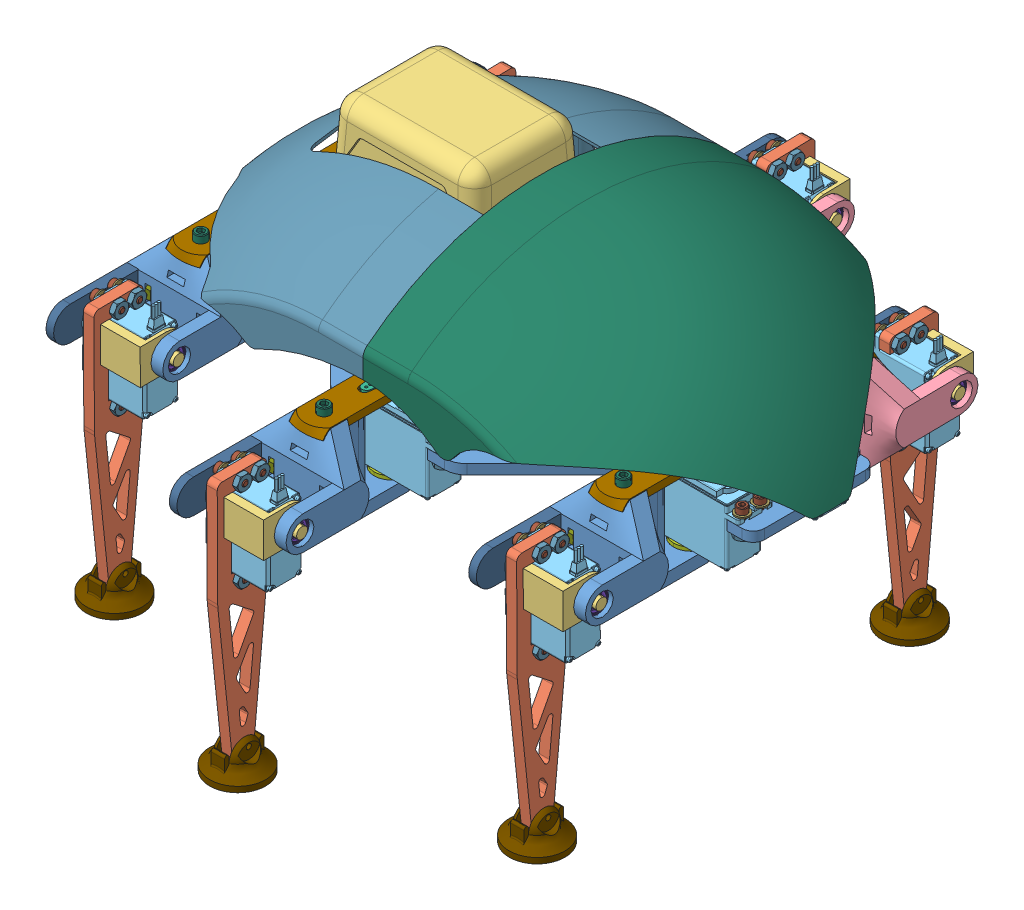
SolidWorks assembly Hexapod_(Leg_V1+Body_V2), configuration Défaut. Lengths in mm. (continued)
Components (placement in the parent): (continued)
- Battery-1: Battery [Défaut] at (-118.1821 62.8376 15.5603) x (0 0 -1) z (-1 0 0) size (64.47 74.3 85.78)
  - MAKITA 4.0AH-1: MAKITA 4.0AH [Défaut] at (0.5853 -29.7874 85.4436) size (64.47 57.15 85.78)
  - MAKITA 4.0AH MOBILE-1: MAKITA 4.0AH MOBILE [Défaut] at (0.5853 -39.3124 91.7936) size (45.84 26.68 66.29)
- arduinoMega-1: arduinoMega [Detailed] at (-199.11 -7.6 14.62) x (0 0 -1) z (-1 0 0) size (108.32 14.5 53.3)
- raspberryPi3B-1: raspberryPi3B [Detailed] at (-109 6.35 15) x (-1 0 0) z (0 1 0) size (87.05 58.5 19.5)
- 12Channel PWM-1: 12Channel PWM [Default] at (-145.6 -5.6 15) x (-1 0 0) z (0 0 1) size (25.4 7.55 66.7)
- DROK_090483.stp-1: DROK_090483.stp [Default] at (-77.5 -5.6 45) x (-1 0 0) z (0 -1 0) size (50.02 60 18.9)
- HX-SHCS 0.138-32x0.625x0.625-N-2: HX-SHCS 0.138-32x0.625x0.625-N [HX-SHCS 0.138-32x0.625x0.625-N] at (-40.288 3.5052 19.09) x (0 -1 0) z (1 0 0) size (19.38 5.74 5.74)
- HX-SHCS 0.138-32x0.625x0.625-N-3: HX-SHCS 0.138-32x0.625x0.625-N [HX-SHCS 0.138-32x0.625x0.625-N] at (-50.288 3.5052 19.09) x (0 -1 0) z (0.5 0 0.866025) size (19.38 5.74 5.74)
- HX-SHCS 0.138-32x0.625x0.625-N-4: HX-SHCS 0.138-32x0.625x0.625-N [HX-SHCS 0.138-32x0.625x0.625-N] at (-50.288 3.5052 10.91) x (0 -1 0) z (1 0 0) size (19.38 5.74 5.74)
- HX-SHCS 0.138-32x0.625x0.625-N-5: HX-SHCS 0.138-32x0.625x0.625-N [HX-SHCS 0.138-32x0.625x0.625-N] at (-40.288 3.5052 10.91) x (0 -1 0) z (1 0 0) size (19.38 5.74 5.74)
- HX-SHCS 0.138-32x0.625x0.625-N-6: HX-SHCS 0.138-32x0.625x0.625-N [HX-SHCS 0.138-32x0.625x0.625-N] at (-170.288 3.5052 69.09) x (0 -1 0) z (1 0 0) size (19.38 5.74 5.74)
- HX-SHCS 0.138-32x0.625x0.625-N-7: HX-SHCS 0.138-32x0.625x0.625-N [HX-SHCS 0.138-32x0.625x0.625-N] at (-160.288 3.5052 69.09) x (0 -1 0) z (1 0 0) size (19.38 5.74 5.74)
- HX-SHCS 0.138-32x0.625x0.625-N-14: HX-SHCS 0.138-32x0.625x0.625-N [HX-SHCS 0.138-32x0.625x0.625-N] at (-160.288 3.5052 -39.09) x (0 -1 0) z (1 0 0) size (19.38 5.74 5.74)
- HX-SHCS 0.138-32x0.625x0.625-N-15: HX-SHCS 0.138-32x0.625x0.625-N [HX-SHCS 0.138-32x0.625x0.625-N] at (-170.288 3.5052 -39.09) x (0 -1 0) z (1 0 0) size (19.38 5.74 5.74)
- HX-SHCS 0.138-32x0.625x0.625-N-16: HX-SHCS 0.138-32x0.625x0.625-N [HX-SHCS 0.138-32x0.625x0.625-N] at (-280.288 3.5052 19.09) x (0 -1 0) z (1 0 0) size (19.38 5.74 5.74)
- HX-SHCS 0.138-32x0.625x0.625-N-17: HX-SHCS 0.138-32x0.625x0.625-N [HX-SHCS 0.138-32x0.625x0.625-N] at (-290.288 3.5052 19.09) x (0 -1 0) z (0.5 0 0.866025) size (19.38 5.74 5.74)
- HX-SHCS 0.138-32x0.625x0.625-N-18: HX-SHCS 0.138-32x0.625x0.625-N [HX-SHCS 0.138-32x0.625x0.625-N] at (-290.288 3.5052 10.91) x (0 -1 0) z (1 0 0) size (19.38 5.74 5.74)
- HX-SHCS 0.138-32x0.625x0.625-N-19: HX-SHCS 0.138-32x0.625x0.625-N [HX-SHCS 0.138-32x0.625x0.625-N] at (-280.288 3.5052 10.91) x (0 -1 0) z (1 0 0) size (19.38 5.74 5.74)
- MSHXNUT 0.138-32-D-N-60: MSHXNUT 0.138-32-D-N [MSHXNUT 0.138-32-D-N] at (-298.75 -8.4956 -15.08) x (1 0 0) z (0 -1 0) size (7.92 9.15 2.9)
- MSHXNUT 0.138-32-D-N-65: MSHXNUT 0.138-32-D-N [MSHXNUT 0.138-32-D-N] at (-298.75 -8.4956 -4.92) x (1 0 0) z (0 -1 0) size (7.92 9.15 2.9)
- MSHXNUT 0.138-32-D-N-70: MSHXNUT 0.138-32-D-N [MSHXNUT 0.138-32-D-N] at (-251.252 -8.4956 -4.92) x (0.5 0 0.866025) z (0 -1 0) size (7.92 9.15 2.9)
- MSHXNUT 0.138-32-D-N-75: MSHXNUT 0.138-32-D-N [MSHXNUT 0.138-32-D-N] at (-251.252 -8.4956 -15.08) x (0.5 0 0.866025) z (0 -1 0) size (7.92 9.15 2.9)
- MSHXNUT 0.138-32-D-N-80: MSHXNUT 0.138-32-D-N [MSHXNUT 0.138-32-D-N] at (-280.288 -13.5656 10.91) x (0 0 1) z (0 -1 0) size (7.92 9.15 2.9)
- MSHXNUT 0.138-32-D-N-85: MSHXNUT 0.138-32-D-N [MSHXNUT 0.138-32-D-N] at (-290.288 -13.5656 10.91) x (0 0 1) z (0 -1 0) size (7.92 9.15 2.9)
- MSHXNUT 0.138-32-D-N-88: MSHXNUT 0.138-32-D-N [MSHXNUT 0.138-32-D-N] at (-178.75 -8.4956 -65.08) x (1 0 0) z (0 -1 0) size (7.92 9.15 2.9)
- MSHXNUT 0.138-32-D-N-89: MSHXNUT 0.138-32-D-N [MSHXNUT 0.138-32-D-N] at (-178.75 -8.4956 -54.92) x (1 0 0) z (0 -1 0) size (7.92 9.15 2.9)
- MSHXNUT 0.138-32-D-N-90: MSHXNUT 0.138-32-D-N [MSHXNUT 0.138-32-D-N] at (-131.252 -8.4956 -54.92) x (0.5 0 0.866025) z (0 -1 0) size (7.92 9.15 2.9)
- MSHXNUT 0.138-32-D-N-91: MSHXNUT 0.138-32-D-N [MSHXNUT 0.138-32-D-N] at (-131.252 -8.4956 -65.08) x (0.5 0 0.866025) z (0 -1 0) size (7.92 9.15 2.9)
- MSHXNUT 0.138-32-D-N-92: MSHXNUT 0.138-32-D-N [MSHXNUT 0.138-32-D-N] at (-160.288 -13.5656 -39.09) x (0 0 1) z (0 -1 0) size (7.92 9.15 2.9)
- MSHXNUT 0.138-32-D-N-93: MSHXNUT 0.138-32-D-N [MSHXNUT 0.138-32-D-N] at (-170.288 -13.5656 -39.09) x (0 0 1) z (0 -1 0) size (7.92 9.15 2.9)
- MSHXNUT 0.138-32-D-N-94: MSHXNUT 0.138-32-D-N [MSHXNUT 0.138-32-D-N] at (-50.288 -13.5656 10.91) x (0 0 1) z (0 -1 0) size (7.92 9.15 2.9)
- MSHXNUT 0.138-32-D-N-95: MSHXNUT 0.138-32-D-N [MSHXNUT 0.138-32-D-N] at (-40.288 -13.5656 10.91) x (0 0 1) z (0 -1 0) size (7.92 9.15 2.9)
- MSHXNUT 0.138-32-D-N-96: MSHXNUT 0.138-32-D-N [MSHXNUT 0.138-32-D-N] at (-11.252 -8.4956 -4.92) x (0.5 0 0.866025) z (0 -1 0) size (7.92 9.15 2.9)
- MSHXNUT 0.138-32-D-N-97: MSHXNUT 0.138-32-D-N [MSHXNUT 0.138-32-D-N] at (-11.252 -8.4956 -15.08) x (0.5 0 0.866025) z (0 -1 0) size (7.92 9.15 2.9)
- MSHXNUT 0.138-32-D-N-98: MSHXNUT 0.138-32-D-N [MSHXNUT 0.138-32-D-N] at (-58.75 -8.4956 -4.92) x (1 0 0) z (0 -1 0) size (7.92 9.15 2.9)
- MSHXNUT 0.138-32-D-N-99: MSHXNUT 0.138-32-D-N [MSHXNUT 0.138-32-D-N] at (-58.75 -8.4956 -15.08) x (1 0 0) z (0 -1 0) size (7.92 9.15 2.9)
- MSHXNUT 0.138-32-D-N-100: MSHXNUT 0.138-32-D-N [MSHXNUT 0.138-32-D-N] at (-290.288 -10.67 19.09) x (0 0 -1) z (0 1 0) size (7.92 9.15 2.9)
- MSHXNUT 0.138-32-D-N-101: MSHXNUT 0.138-32-D-N [MSHXNUT 0.138-32-D-N] at (-280.288 -10.67 19.09) x (0 0 -1) z (0 1 0) size (7.92 9.15 2.9)
- MSHXNUT 0.138-32-D-N-102: MSHXNUT 0.138-32-D-N [MSHXNUT 0.138-32-D-N] at (-251.252 -5.6 34.92) x (0.5 0 -0.866025) z (0 1 0) size (7.92 9.15 2.9)
- MSHXNUT 0.138-32-D-N-103: MSHXNUT 0.138-32-D-N [MSHXNUT 0.138-32-D-N] at (-251.252 -5.6 45.08) x (0.5 0 -0.866025) z (0 1 0) size (7.92 9.15 2.9)
- MSHXNUT 0.138-32-D-N-104: MSHXNUT 0.138-32-D-N [MSHXNUT 0.138-32-D-N] at (-298.75 -5.6 34.92) x (1 0 0) z (0 1 0) size (7.92 9.15 2.9)
- MSHXNUT 0.138-32-D-N-105: MSHXNUT 0.138-32-D-N [MSHXNUT 0.138-32-D-N] at (-298.75 -5.6 45.08) x (1 0 0) z (0 1 0) size (7.92 9.15 2.9)
- MSHXNUT 0.138-32-D-N-106: MSHXNUT 0.138-32-D-N [MSHXNUT 0.138-32-D-N] at (-178.75 -5.6 95.08) x (1 0 0) z (0 1 0) size (7.92 9.15 2.9)
- MSHXNUT 0.138-32-D-N-107: MSHXNUT 0.138-32-D-N [MSHXNUT 0.138-32-D-N] at (-178.75 -5.6 84.92) x (1 0 0) z (0 1 0) size (7.92 9.15 2.9)
- MSHXNUT 0.138-32-D-N-108: MSHXNUT 0.138-32-D-N [MSHXNUT 0.138-32-D-N] at (-131.252 -5.6 84.92) x (0.5 0 -0.866025) z (0 1 0) size (7.92 9.15 2.9)
- MSHXNUT 0.138-32-D-N-109: MSHXNUT 0.138-32-D-N [MSHXNUT 0.138-32-D-N] at (-131.252 -5.6 95.08) x (0.5 0 -0.866025) z (0 1 0) size (7.92 9.15 2.9)
- MSHXNUT 0.138-32-D-N-110: MSHXNUT 0.138-32-D-N [MSHXNUT 0.138-32-D-N] at (-160.288 -10.67 69.09) x (0 0 -1) z (0 1 0) size (7.92 9.15 2.9)
- MSHXNUT 0.138-32-D-N-111: MSHXNUT 0.138-32-D-N [MSHXNUT 0.138-32-D-N] at (-170.288 -10.67 69.09) x (0 0 -1) z (0 1 0) size (7.92 9.15 2.9)
- MSHXNUT 0.138-32-D-N-112: MSHXNUT 0.138-32-D-N [MSHXNUT 0.138-32-D-N] at (-50.288 -10.67 19.09) x (0 0 -1) z (0 1 0) size (7.92 9.15 2.9)
- MSHXNUT 0.138-32-D-N-113: MSHXNUT 0.138-32-D-N [MSHXNUT 0.138-32-D-N] at (-40.288 -10.67 19.09) x (0 0 -1) z (0 1 0) size (7.92 9.15 2.9)
- MSHXNUT 0.138-32-D-N-114: MSHXNUT 0.138-32-D-N [MSHXNUT 0.138-32-D-N] at (-11.252 -5.6 34.92) x (0.5 0 -0.866025) z (0 1 0) size (7.92 9.15 2.9)
- MSHXNUT 0.138-32-D-N-115: MSHXNUT 0.138-32-D-N [MSHXNUT 0.138-32-D-N] at (-11.252 -5.6 45.08) x (0.5 0 -0.866025) z (0 1 0) size (7.92 9.15 2.9)
- MSHXNUT 0.138-32-D-N-116: MSHXNUT 0.138-32-D-N [MSHXNUT 0.138-32-D-N] at (-58.75 -5.6 34.92) x (1 0 0) z (0 1 0) size (7.92 9.15 2.9)
- MSHXNUT 0.138-32-D-N-117: MSHXNUT 0.138-32-D-N [MSHXNUT 0.138-32-D-N] at (-58.75 -5.6 45.08) x (1 0 0) z (0 1 0) size (7.92 9.15 2.9)
- HX-SHCS 0.138-32x0.5x0.5-N-20: HX-SHCS 0.138-32x0.5x0.5-N [HX-SHCS 0.138-32x0.5x0.5-N] at (-175 -12.6052 48.88) x (0 1 0) z (-0.5 0 -0.866025) size (16.21 5.74 5.74)
- HX-SHCS 0.138-32x0.5x0.5-N-21: HX-SHCS 0.138-32x0.5x0.5-N [HX-SHCS 0.138-32x0.5x0.5-N] at (-223.22 -12.6052 -32.36) x (0 1 0) z (1 0 0) size (16.21 5.74 5.74)
- HX-SHCS 0.138-32x0.5x0.5-N-22: HX-SHCS 0.138-32x0.5x0.5-N [HX-SHCS 0.138-32x0.5x0.5-N] at (-175 -12.6052 -26) x (0 1 0) z (-0.5 0 -0.866025) size (16.21 5.74 5.74)
- HX-SHCS 0.138-32x0.5x0.5-N-23: HX-SHCS 0.138-32x0.5x0.5-N [HX-SHCS 0.138-32x0.5x0.5-N] at (-223.22 -12.6052 50.11) x (0 1 0) z (-1 0 0) size (16.21 5.74 5.74)
- MSHXNUT 0.112-40-D-N-106: MSHXNUT 0.112-40-D-N [MSHXNUT 0.112-40-D-N] at (-223.22 2.4892 -32.36) x (1 0 0) z (0 1 0) size (6.35 7.33 2.49)
- MSHXNUT 0.112-40-D-N-107: MSHXNUT 0.112-40-D-N [MSHXNUT 0.112-40-D-N] at (-223.22 2.4892 50.11) x (1 0 0) z (0 1 0) size (6.35 7.33 2.49)
- MSHXNUT 0.112-40-D-N-108: MSHXNUT 0.112-40-D-N [MSHXNUT 0.112-40-D-N] at (-175 2.4892 -26) x (1 0 0) z (0 1 0) size (6.35 7.33 2.49)
- MSHXNUT 0.112-40-D-N-109: MSHXNUT 0.112-40-D-N [MSHXNUT 0.112-40-D-N] at (-175 2.4892 48.88) x (1 0 0) z (0 1 0) size (6.35 7.33 2.49)
- HX-SHCS 0.138-32x0.5x0.5-N-24: HX-SHCS 0.138-32x0.5x0.5-N [HX-SHCS 0.138-32x0.5x0.5-N] at (-117.315 -10.3052 -11.415) x (0 1 0) z (-0.5 0 -0.866025) size (16.21 5.74 5.74)
- MSHXNUT 0.112-40-D-N-110: MSHXNUT 0.112-40-D-N [MSHXNUT 0.112-40-D-N] at (-117.315 2.4892 -11.415) x (1 0 0) z (0 1 0) size (6.35 7.33 2.49)
- HX-SHCS 0.138-32x0.5x0.5-N-28: HX-SHCS 0.138-32x0.5x0.5-N [HX-SHCS 0.138-32x0.5x0.5-N] at (-80.685 -10.3052 -11.415) x (0 1 0) z (-0.5 0 -0.866025) size (16.21 5.74 5.74)
- HX-SHCS 0.138-32x0.5x0.5-N-29: HX-SHCS 0.138-32x0.5x0.5-N [HX-SHCS 0.138-32x0.5x0.5-N] at (-117.315 -10.3052 41.415) x (0 1 0) z (-0.5 0 -0.866025) size (16.21 5.74 5.74)
- HX-SHCS 0.138-32x0.5x0.5-N-30: HX-SHCS 0.138-32x0.5x0.5-N [HX-SHCS 0.138-32x0.5x0.5-N] at (-80.685 -10.3052 41.415) x (0 1 0) z (-0.5 0 -0.866025) size (16.21 5.74 5.74)
- MSHXNUT 0.112-40-D-N-114: MSHXNUT 0.112-40-D-N [MSHXNUT 0.112-40-D-N] at (-80.685 2.4892 -11.415) x (1 0 0) z (0 1 0) size (6.35 7.33 2.49)
- MSHXNUT 0.112-40-D-N-115: MSHXNUT 0.112-40-D-N [MSHXNUT 0.112-40-D-N] at (-117.315 2.4892 41.415) x (1 0 0) z (0 1 0) size (6.35 7.33 2.49)
- MSHXNUT 0.112-40-D-N-116: MSHXNUT 0.112-40-D-N [MSHXNUT 0.112-40-D-N] at (-80.685 2.4892 41.415) x (1 0 0) z (0 1 0) size (6.35 7.33 2.49)
- 1_4_Round_Aluminum_Standoff.step-1: 1_4_Round_Aluminum_Standoff.step [Défaut] at (-70 0 -9.5) x (0.963282 0 -0.268492) z (0.268492 0 0.963282) size (6.34 6.36 6.34)
- HX-SHCS 0.112-40x1x0.75-N-28: HX-SHCS 0.112-40x1x0.75-N [HX-SHCS 0.112-40x1x0.75-N] at (-70 10.4948 -9.5) x (0 -1 0) z (0.637638 0 0.770336) size (28.24 4.65 4.65)
- MSHXNUT 0.112-40-D-N-117: MSHXNUT 0.112-40-D-N [MSHXNUT 0.112-40-D-N] at (-70 -8.0892 -9.5) x (1 0 0) z (0 -1 0) size (6.35 7.33 2.49)
- 1_4_Round_Aluminum_Standoff.step-2: 1_4_Round_Aluminum_Standoff.step [Défaut] at (-128 0 -9.5) x (0.963282 0 -0.268492) z (0.268492 0 0.963282) size (6.34 6.36 6.34)
- 1_4_Round_Aluminum_Standoff.step-3: 1_4_Round_Aluminum_Standoff.step [Défaut] at (-70 0 39.5) x (0.963282 0 -0.268492) z (0.268492 0 0.963282) size (6.34 6.36 6.34)
- 1_4_Round_Aluminum_Standoff.step-4: 1_4_Round_Aluminum_Standoff.step [Défaut] at (-128 0 39.5) x (0.963282 0 -0.268492) z (0.268492 0 0.963282) size (6.34 6.36 6.34)
- MSHXNUT 0.112-40-D-N-121: MSHXNUT 0.112-40-D-N [MSHXNUT 0.112-40-D-N] at (-128 -8.0892 -9.5) x (1 0 0) z (0 -1 0) size (6.35 7.33 2.49)
- MSHXNUT 0.112-40-D-N-122: MSHXNUT 0.112-40-D-N [MSHXNUT 0.112-40-D-N] at (-70 -8.0892 39.5) x (1 0 0) z (0 -1 0) size (6.35 7.33 2.49)
- MSHXNUT 0.112-40-D-N-123: MSHXNUT 0.112-40-D-N [MSHXNUT 0.112-40-D-N] at (-128 -8.0892 39.5) x (1 0 0) z (0 -1 0) size (6.35 7.33 2.49)
- HX-SHCS 0.112-40x1x0.75-N-32: HX-SHCS 0.112-40x1x0.75-N [HX-SHCS 0.112-40x1x0.75-N] at (-128 10.4948 -9.5) x (0 -1 0) z (0.637638 0 0.770336) size (28.24 4.65 4.65)
- HX-SHCS 0.112-40x1x0.75-N-33: HX-SHCS 0.112-40x1x0.75-N [HX-SHCS 0.112-40x1x0.75-N] at (-70 10.4948 39.5) x (0 -1 0) z (0.637638 0 0.770336) size (28.24 4.65 4.65)
- HX-SHCS 0.112-40x1x0.75-N-34: HX-SHCS 0.112-40x1x0.75-N [HX-SHCS 0.112-40x1x0.75-N] at (-128 10.4948 39.5) x (0 -1 0) z (0.637638 0 0.770336) size (28.24 4.65 4.65)
- HX-SHCS 0.112-40x0.5x0.5-N-32: HX-SHCS 0.112-40x0.5x0.5-N [HX-SHCS 0.112-40x0.5x0.5-N] at (-155 -9.9448 -12.95) x (0 1 0) z (-1 0 0) size (15.54 4.65 4.65)
- MSHXNUT 0.112-40-D-N-124: MSHXNUT 0.112-40-D-N [MSHXNUT 0.112-40-D-N] at (-155 2.4892 -12.95) x (1 0 0) z (0 1 0) size (6.35 7.33 2.49)
- HX-SHCS 0.112-40x0.5x0.5-N-36: HX-SHCS 0.112-40x0.5x0.5-N [HX-SHCS 0.112-40x0.5x0.5-N] at (-136.2 -9.9448 -12.95) x (0 1 0) z (-1 0 0) size (15.54 4.65 4.65)
- HX-SHCS 0.112-40x0.5x0.5-N-37: HX-SHCS 0.112-40x0.5x0.5-N [HX-SHCS 0.112-40x0.5x0.5-N] at (-155 -9.9448 42.95) x (0 1 0) z (-1 0 0) size (15.54 4.65 4.65)
- HX-SHCS 0.112-40x0.5x0.5-N-38: HX-SHCS 0.112-40x0.5x0.5-N [HX-SHCS 0.112-40x0.5x0.5-N] at (-136.2 -9.9448 42.95) x (0 1 0) z (-1 0 0) size (15.54 4.65 4.65)
- MSHXNUT 0.112-40-D-N-128: MSHXNUT 0.112-40-D-N [MSHXNUT 0.112-40-D-N] at (-136.2 2.4892 -12.95) x (1 0 0) z (0 1 0) size (6.35 7.33 2.49)
- MSHXNUT 0.112-40-D-N-129: MSHXNUT 0.112-40-D-N [MSHXNUT 0.112-40-D-N] at (-155 2.4892 42.95) x (1 0 0) z (0 1 0) size (6.35 7.33 2.49)
- MSHXNUT 0.112-40-D-N-130: MSHXNUT 0.112-40-D-N [MSHXNUT 0.112-40-D-N] at (-136.2 2.4892 42.95) x (1 0 0) z (0 1 0) size (6.35 7.33 2.49)
- 1_4_Round_Aluminum_Standoff.step-5: 1_4_Round_Aluminum_Standoff.step [Défaut] at (-174 0 -7) x (0.963282 0 -0.268492) z (0.268492 0 0.963282) size (6.34 6.36 6.34)
- 1_4_Round_Aluminum_Standoff.step-6: 1_4_Round_Aluminum_Standoff.step [Défaut] at (-174 0 37) x (0.963282 0 -0.268492) z (0.268492 0 0.963282) size (6.34 6.36 6.34)
- 1_4_Round_Aluminum_Standoff.step-7: 1_4_Round_Aluminum_Standoff.step [Défaut] at (-240 0 -7) x (0.963282 0 -0.268492) z (0.268492 0 0.963282) size (6.34 6.36 6.34)
- 1_4_Round_Aluminum_Standoff.step-8: 1_4_Round_Aluminum_Standoff.step [Défaut] at (-240 0 37) x (0.963282 0 -0.268492) z (0.268492 0 0.963282) size (6.34 6.36 6.34)
- HX-SHCS 0.112-40x1x0.75-N-40: HX-SHCS 0.112-40x1x0.75-N [HX-SHCS 0.112-40x1x0.75-N] at (-174 -8.4448 -7) x (0 1 0) z (-0.415316 0 -0.909677) size (28.24 4.65 4.65)
- HX-SHCS 0.112-40x1x0.75-N-44: HX-SHCS 0.112-40x1x0.75-N [HX-SHCS 0.112-40x1x0.75-N] at (-174 -8.4448 37) x (0 1 0) z (-0.415316 0 -0.909677) size (28.24 4.65 4.65)
- HX-SHCS 0.112-40x1x0.75-N-45: HX-SHCS 0.112-40x1x0.75-N [HX-SHCS 0.112-40x1x0.75-N] at (-240 -8.4448 -7) x (0 1 0) z (-0.415316 0 -0.909677) size (28.24 4.65 4.65)
- HX-SHCS 0.112-40x1x0.75-N-46: HX-SHCS 0.112-40x1x0.75-N [HX-SHCS 0.112-40x1x0.75-N] at (-240 -8.4448 37) x (0 1 0) z (-0.415316 0 -0.909677) size (28.24 4.65 4.65)
- Batterie_holder-1: Batterie_holder [Default] at (-223 17.7 15) size (72 19.6 50)
- MSHXNUT 0.112-40-D-N-131: MSHXNUT 0.112-40-D-N [MSHXNUT 0.112-40-D-N] at (-174 15.1892 -7) x (1 0 0) z (0 1 0) size (6.35 7.33 2.49)
- MSHXNUT 0.112-40-D-N-135: MSHXNUT 0.112-40-D-N [MSHXNUT 0.112-40-D-N] at (-174 15.1892 37) x (1 0 0) z (0 1 0) size (6.35 7.33 2.49)
- MSHXNUT 0.112-40-D-N-136: MSHXNUT 0.112-40-D-N [MSHXNUT 0.112-40-D-N] at (-240 15.1892 -7) x (1 0 0) z (0 1 0) size (6.35 7.33 2.49)
- MSHXNUT 0.112-40-D-N-137: MSHXNUT 0.112-40-D-N [MSHXNUT 0.112-40-D-N] at (-240 15.1892 37) x (1 0 0) z (0 1 0) size (6.35 7.33 2.49)
- Shell_(Front)-3: Shell_(Front) [Default] at (-155 -76.2 15) x (0 0 1) z (-1 0 0) size (204.71 79.03 165.14)
- Shell_(Back)-3: Shell_(Back) [Default] at (-155 -76.2 15) x (0 0 -1) z (1 0 0) size (205.09 91.22 173.55)
Mates (geometry in assembly coordinates):
- Coincident2: coincident anti-aligned: plane of Body_V2-5 through (-295 -5.601 0) normal (0 0 -1)
- Coincident3: coincident aligned: plane of Body_V2-5 through (-310 0 15) normal (0 1 0)
- Coincident4: coincident aligned: plane of Body_V2-5 through (0 0 50) normal (1 0 0)
- Coincident5: coincident anti-aligned: plane of Body_V2-5 through (-310 0 15) normal (0 1 0); plane of Leg-6/hs-422-3 through (-35.001 0 -0.094) normal (0 -1 0)
- Concentric3: concentric anti-aligned: cylinder of Body_V2-5 through (-58.75 0 -15.08) axis (0 -1 0) radius 1.45; cylinder of Leg-6/hs-422-3 through (-58.75 -26.67 -15.08) axis (0 1 0) radius 2.1844
- Concentric6: concentric aligned: cylinder of Body_V2-5 through (-298.75 -5.601 -4.92) axis (0 1 0) radius 1.45; cylinder of Leg-7/hs-422-3 through (-298.75 -26.67 -4.92) axis (0 1 0) radius 2.1844
- Parallel4: parallel anti-aligned: plane of Body_V2-5 through (-295 -5.601 0) normal (0 0 -1); plane of Leg-7/hs-422-3 through (-275.001 -5.969 -0.094) normal (0 0 1)
- Coincident9: coincident anti-aligned: plane of Body_V2-5 through (-310 0 15) normal (0 1 0); plane of Leg-7/hs-422-3 through (-275.001 0 -0.094) normal (0 -1 0)
- Coincident10: coincident anti-aligned: plane of Body_V2-5 through (-310 0 15) normal (0 1 0); plane of Leg-8/hs-422-3 through (-155.001 0 -50.094) normal (0 -1 0)
- Concentric7: concentric anti-aligned: cylinder of Body_V2-5 through (-178.75 0 -54.92) axis (0 -1 0) radius 1.45; cylinder of Leg-8/hs-422-3 through (-178.75 -26.67 -54.92) axis (0 1 0) radius 2.1844
- Parallel5: parallel anti-aligned: plane of Body_V2-5 through (-175 -5.6 -50) normal (0 0 -1); plane of Leg-8/hs-422-3 through (-155.001 -5.969 -50.094) normal (0 0 1)
- Parallel6: parallel anti-aligned: plane of Body_V2-5 through (-55 -5.6 0) normal (0 0 -1); plane of Leg-6/hs-422-3 through (-35.001 -5.969 -0.094) normal (0 0 1)
- Coincident11: coincident anti-aligned: plane of Body_V2-5 through (-310 0 15) normal (0 1 0); plane of Leg_(Straight_Foot)_(Mirror)-4/hs-422-3 through (-275.001 0 49.906) normal (0 -1 0)
- Concentric8: concentric aligned: cylinder of Body_V2-5 through (-298.75 -5.601 45.08) axis (0 1 0) radius 1.45; cylinder of Leg_(Straight_Foot)_(Mirror)-4/hs-422-3 through (-298.75 -26.67 45.08) axis (0 1 0) radius 2.1844
- Parallel7: parallel anti-aligned: plane of Body_V2-5 through (-295 -5.601 30) normal (0 0 1); plane of Leg_(Straight_Foot)_(Mirror)-4/hs-422-3 through (-275.001 -5.969 30.094) normal (0 0 -1)
- Coincident13: coincident anti-aligned: plane of Body_V2-5 through (-310 0 15) normal (0 1 0); plane of Leg_(Straight_Foot)_(Mirror)-5/hs-422-3 through (-35.001 0 49.906) normal (0 -1 0)
- Concentric9: concentric anti-aligned: cylinder of Body_V2-5 through (-58.75 0 45.08) axis (0 -1 0) radius 1.45; cylinder of Leg_(Straight_Foot)_(Mirror)-5/hs-422-3 through (-58.75 -26.67 45.08) axis (0 1 0) radius 2.1844
- Parallel8: parallel anti-aligned: plane of Body_V2-5 through (-55 -5.6 30) normal (0 0 1); plane of Leg_(Straight_Foot)_(Mirror)-5/hs-422-3 through (-35.001 -5.969 30.094) normal (0 0 -1)
- Coincident15: coincident anti-aligned: plane of Body_V2-5 through (-310 0 15) normal (0 1 0); plane of Leg_(Straight_Foot)_(Mirror)-6/hs-422-3 through (-155.001 0 99.906) normal (0 -1 0)
- Concentric10: concentric anti-aligned: cylinder of Body_V2-5 through (-178.75 0 95.08) axis (0 -1 0) radius 1.45; cylinder of Leg_(Straight_Foot)_(Mirror)-6/hs-422-3 through (-178.75 -26.67 95.08) axis (0 1 0) radius 2.1844
- Parallel9: parallel anti-aligned: plane of Body_V2-5 through (-175 -5.6 80) normal (0 0 1); plane of Leg_(Straight_Foot)_(Mirror)-6/hs-422-3 through (-155.001 -5.969 80.094) normal (0 0 -1)
- Coïncidente2: coincident anti-aligned: plane of arduinoMega-1 through (-199.11 -5.6 14.62) normal (0 1 0); plane of Body_V2-5 through (-310 -5.6 15) normal (0 -1 0)
- Coïncidente4: coincident anti-aligned: plane of Body_V2-5 through (-310 -5.6 15) normal (0 -1 0); plane of 12Channel PWM-1 through (-155 -5.6 -12.95) normal (0 1 0)
- Coïncidente5: coincident anti-aligned: plane of Body_V2-5 through (-310 -5.6 15) normal (0 -1 0); plane of DROK_090483.stp-1 through (-99 -5.6 15) normal (0 1 0)
- Parallèle4: parallel aligned: plane of Body_V2-5 through (0 0 50) normal (1 0 0); plane of 12Channel PWM-1 through (-132.9 -7.1 -12.95) normal (1 0 0)
- Concentric13: concentric aligned: cylinder of Body_V2-5 through (-155 0 42.95) axis (0 -1 0) radius 1.25; cylinder of 12Channel PWM-1 through (-155 -2.0645 42.95) axis (0 -1 0) radius 1.25
- Concentric17: concentric anti-aligned: circle of Body-1; circle of DROK_090483.stp-1
- Concentric18: concentric aligned: cylinder of Body_V2-5 through (-80.685 0 41.415) axis (0 -1 0) radius 1.45; cylinder of DROK_090483.stp-1 through (-80.685 -5.6 41.415) axis (0 -1 0) radius 1.585
- Concentric19: concentric aligned: cylinder of Body_V2-5 through (-175 0 -26) axis (0 -1 0) radius 1.6; circle of arduinoMega-1
- Concentric22: concentric aligned: cylinder of Body_V2-5 through (-223.22 0 50.11) axis (0 -1 0) radius 1.6; cylinder of arduinoMega-1 through (-223.22 -7.6 50.11) axis (0 -1 0) radius 1.6
- Concentric23: concentric anti-aligned: cylinder of Body_V2-5 through (-40.288 0 19.09) axis (0 -1 0) radius 1.45; cylinder of HX-SHCS 0.138-32x0.625x0.625-N-2 through (-40.288 35.2552 19.09) axis (0 1 0) radius 1.7526
- Concentric24: concentric anti-aligned: cylinder of Body_V2-5 through (-50.288 0 19.09) axis (0 -1 0) radius 1.45; cylinder of HX-SHCS 0.138-32x0.625x0.625-N-3 through (-50.288 35.2552 19.09) axis (0 1 0) radius 1.7526
- Coincident19: coincident anti-aligned: plane of Body_V2-5 through (-310 0 15) normal (0 1 0); plane of HX-SHCS 0.138-32x0.625x0.625-N-2 through (-40.288 0 16.2198) normal (0 -1 0)
- Coincident20: coincident anti-aligned: plane of Body_V2-5 through (-310 0 15) normal (0 1 0); plane of HX-SHCS 0.138-32x0.625x0.625-N-3 through (-47.8023 0 17.6549) normal (0 -1 0)
- Parallel10: parallel aligned: plane of Body_V2-5 through (0 0 50) normal (1 0 0); plane of HX-SHCS 0.138-32x0.625x0.625-N-3 through (-51.6723 1.8796 19.8892) normal (1 0 0)
- Parallel11: parallel aligned: plane of Body_V2-5 through (0 0 50) normal (1 0 0); plane of HX-SHCS 0.138-32x0.625x0.625-N-2 through (-41.6723 1.8796 18.2908) normal (1 0 0)
- Concentric25: concentric anti-aligned: cylinder of Body_V2-5 through (-50.288 0 10.91) axis (0 -1 0) radius 1.45; cylinder of HX-SHCS 0.138-32x0.625x0.625-N-4 through (-50.288 35.2552 10.91) axis (0 1 0) radius 1.7526
- Concentric26: concentric anti-aligned: cylinder of Body_V2-5 through (-40.288 0 10.91) axis (0 -1 0) radius 1.45; cylinder of HX-SHCS 0.138-32x0.625x0.625-N-5 through (-40.288 35.2552 10.91) axis (0 1 0) radius 1.7526
- Coincident23: coincident anti-aligned: plane of Body_V2-5 through (-310 0 15) normal (0 1 0); plane of HX-SHCS 0.138-32x0.625x0.625-N-5 through (-40.288 0 8.0398) normal (0 -1 0)
- Coincident24: coincident anti-aligned: plane of Body_V2-5 through (-310 0 15) normal (0 1 0); plane of HX-SHCS 0.138-32x0.625x0.625-N-4 through (-50.288 0 8.0398) normal (0 -1 0)
- Parallel12: parallel aligned: plane of Body_V2-5 through (0 0 50) normal (1 0 0); plane of HX-SHCS 0.138-32x0.625x0.625-N-5 through (-41.6723 1.8796 10.1108) normal (1 0 0)
- Parallel13: parallel aligned: plane of Body_V2-5 through (0 0 50) normal (1 0 0); plane of HX-SHCS 0.138-32x0.625x0.625-N-4 through (-51.6723 1.8796 10.1108) normal (1 0 0)
- Concentric27: concentric anti-aligned: cylinder of Body_V2-5 through (-170.288 0 -39.09) axis (0 -1 0) radius 1.45; cylinder of HX-SHCS 0.138-32x0.625x0.625-N-13 through (-214.94 40.2807 -39.09) axis (0 1 0) radius 1.7526
- Concentric29: concentric anti-aligned: cylinder of Body_V2-5 through (-160.288 0 69.09) axis (0 -1 0) radius 1.45; cylinder of HX-SHCS 0.138-32x0.625x0.625-N-7 through (-160.288 35.2552 69.09) axis (0 1 0) radius 1.7526
- Concentric30: concentric anti-aligned: cylinder of Body_V2-5 through (-170.288 0 69.09) axis (0 -1 0) radius 1.45; cylinder of HX-SHCS 0.138-32x0.625x0.625-N-6 through (-170.288 35.2552 69.09) axis (0 1 0) radius 1.7526
- Coincident27: coincident anti-aligned: plane of Body_V2-5 through (-310 0 15) normal (0 1 0); plane of HX-SHCS 0.138-32x0.625x0.625-N-7 through (-160.288 0 66.2198) normal (0 -1 0)
- Coincident28: coincident anti-aligned: plane of Body_V2-5 through (-310 0 15) normal (0 1 0); plane of HX-SHCS 0.138-32x0.625x0.625-N-6 through (-170.288 0 66.2198) normal (0 -1 0)
- Parallel14: parallel aligned: plane of Body_V2-5 through (0 0 50) normal (1 0 0); plane of HX-SHCS 0.138-32x0.625x0.625-N-6 through (-171.6723 1.8796 68.2908) normal (1 0 0)
- Parallel15: parallel aligned: plane of Body_V2-5 through (0 0 50) normal (1 0 0); plane of HX-SHCS 0.138-32x0.625x0.625-N-7 through (-161.6723 1.8796 68.2908) normal (1 0 0)
- Concentric31: concentric anti-aligned: cylinder of Body_V2-5 through (-170.288 0 -39.09) axis (0 -1 0) radius 1.45; cylinder of HX-SHCS 0.138-32x0.625x0.625-N-15 through (-170.288 35.2552 -39.09) axis (0 1 0) radius 1.7526
- Concentric32: concentric anti-aligned: cylinder of Body_V2-5 through (-160.288 0 -39.09) axis (0 -1 0) radius 1.45; cylinder of HX-SHCS 0.138-32x0.625x0.625-N-14 through (-160.288 35.2552 -39.09) axis (0 1 0) radius 1.7526
- Coincident31: coincident anti-aligned: plane of Body_V2-5 through (-310 0 15) normal (0 1 0); plane of HX-SHCS 0.138-32x0.625x0.625-N-15 through (-170.288 0 -41.9602) normal (0 -1 0)
- Coincident32: coincident anti-aligned: plane of Body_V2-5 through (-310 0 15) normal (0 1 0); plane of HX-SHCS 0.138-32x0.625x0.625-N-14 through (-160.288 0 -41.9602) normal (0 -1 0)
- Parallel16: parallel anti-aligned: plane of Body_V2-5 through (0 0 50) normal (1 0 0); plane of HX-SHCS 0.138-32x0.625x0.625-N-15 through (-168.9037 1.8796 -38.2908) normal (-1 0 0)
- Parallel17: parallel anti-aligned: plane of Body_V2-5 through (0 0 50) normal (1 0 0); plane of HX-SHCS 0.138-32x0.625x0.625-N-14 through (-158.9037 1.8796 -38.2908) normal (-1 0 0)
- Concentric33: concentric aligned: cylinder of Body_V2-5 through (-290.288 -5.601 19.09) axis (0 1 0) radius 1.45; cylinder of HX-SHCS 0.138-32x0.625x0.625-N-17 through (-290.288 35.2552 19.09) axis (0 1 0) radius 1.7526
- Concentric34: concentric aligned: circle of Body-1; cylinder of HX-SHCS 0.138-32x0.625x0.625-N-16 through (-280.288 35.2552 19.09) axis (0 1 0) radius 1.7526
- Concentric35: concentric aligned: cylinder of Body_V2-5 through (-290.288 -5.601 10.91) axis (0 1 0) radius 1.45; cylinder of HX-SHCS 0.138-32x0.625x0.625-N-18 through (-290.288 35.2552 10.91) axis (0 1 0) radius 1.7526
- Concentric36: concentric aligned: cylinder of Body_V2-5 through (-280.288 -5.601 10.91) axis (0 1 0) radius 1.45; cylinder of HX-SHCS 0.138-32x0.625x0.625-N-19 through (-280.288 35.2552 10.91) axis (0 1 0) radius 1.7526
- Coincident35: coincident anti-aligned: plane of Body_V2-5 through (-310 0 15) normal (0 1 0); plane of HX-SHCS 0.138-32x0.625x0.625-N-18 through (-290.288 0 8.0398) normal (0 -1 0)
- Coincident36: coincident anti-aligned: plane of Body_V2-5 through (-310 0 15) normal (0 1 0); plane of HX-SHCS 0.138-32x0.625x0.625-N-19 through (-280.288 0 8.0398) normal (0 -1 0)
- Coincident37: coincident anti-aligned: plane of Body_V2-5 through (-310 0 15) normal (0 1 0); plane of HX-SHCS 0.138-32x0.625x0.625-N-17 through (-287.8023 0 17.6549) normal (0 -1 0)
- Coincident38: coincident anti-aligned: plane of Body_V2-5 through (-310 0 15) normal (0 1 0); plane of HX-SHCS 0.138-32x0.625x0.625-N-16 through (-280.288 0 16.2198) normal (0 -1 0)
- Parallel18: parallel anti-aligned: plane of Body_V2-5 through (0 0 50) normal (1 0 0); plane of HX-SHCS 0.138-32x0.625x0.625-N-19 through (-278.9037 1.8796 11.7092) normal (-1 0 0)
- Parallel19: parallel anti-aligned: plane of Body_V2-5 through (0 0 50) normal (1 0 0); plane of HX-SHCS 0.138-32x0.625x0.625-N-18 through (-288.9037 1.8796 11.7092) normal (-1 0 0)
- Parallel20: parallel anti-aligned: plane of Body_V2-5 through (0 0 50) normal (1 0 0); plane of HX-SHCS 0.138-32x0.625x0.625-N-16 through (-278.9037 1.8796 19.8892) normal (-1 0 0)
- Parallel21: parallel anti-aligned: plane of Body_V2-5 through (0 0 50) normal (1 0 0); plane of HX-SHCS 0.138-32x0.625x0.625-N-17 through (-288.9037 1.8796 18.2908) normal (-1 0 0)
- Concentric37: concentric anti-aligned: cylinder of Leg_(Straight_Foot)-7/socket_1_2_6-32_with_washer-7/HX-SHCS 0.138-32x0.5x0.5-N-1 through (-298.75 38.5826 -15.08) axis (0 1 0) radius 1.7526; circle of MSHXNUT 0.138-32-D-N-1
- Coincident40: coincident anti-aligned: plane of Body_V2-5 through (-310 -5.6 15) normal (0 -1 0); plane of MSHXNUT 0.138-32-D-N-60 through (-306.6748 -5.6 -15.08) normal (0 1 0)
- Parallel22: parallel aligned: plane of Leg-7/hs-422-3 through (-294.94 -5.969 -0.094) normal (-1 0 0); plane of MSHXNUT 0.138-32-D-N-60 through (-302.7124 -5.6 -12.7923) normal (-1 0 0)
- Concentric38: concentric anti-aligned: cylinder of Leg_(Straight_Foot)-7/socket_1_2_6-32_with_washer-5/HX-SHCS 0.138-32x0.5x0.5-N-1 through (-298.75 38.5826 -4.92) axis (0 1 0) radius 1.7526; circle of MSHXNUT 0.138-32-D-N-2
- Parallel23: parallel aligned: plane of Leg-7/hs-422-3 through (-294.94 -5.969 -0.094) normal (-1 0 0); plane of MSHXNUT 0.138-32-D-N-65 through (-302.7124 -5.6 -2.6323) normal (-1 0 0)
- Coincident44: coincident anti-aligned: plane of Body_V2-5 through (-310 -5.6 15) normal (0 -1 0); plane of MSHXNUT 0.138-32-D-N-65 through (-306.6748 -5.6 -4.92) normal (0 1 0)
- Coincident45: coincident anti-aligned: cylinder of Leg_(Straight_Foot)-7/socket_1_2_6-32_with_washer-8/HX-SHCS 0.138-32x0.5x0.5-N-1 through (-251.252 38.5826 -4.92) axis (0 1 0) radius 1.7526; circle of MSHXNUT 0.138-32-D-N-3
- Concentric40: concentric anti-aligned: cylinder of Leg_(Straight_Foot)-7/socket_1_2_6-32_with_washer-6/HX-SHCS 0.138-32x0.5x0.5-N-1 through (-251.252 38.5826 -15.08) axis (0 1 0) radius 1.7526; circle of MSHXNUT 0.138-32-D-N-4
- Coincident47: coincident anti-aligned: plane of Body_V2-5 through (-310 -5.6 15) normal (0 -1 0); plane of MSHXNUT 0.138-32-D-N-75 through (-255.2144 -5.6 -21.9431) normal (0 1 0)
- Coincident48: coincident anti-aligned: plane of Body_V2-5 through (-310 -5.6 15) normal (0 -1 0); plane of MSHXNUT 0.138-32-D-N-70 through (-255.2144 -5.6 -11.7831) normal (0 1 0)
- Parallel24: parallel aligned: plane of Leg-7/hs-422-3 through (-255.062 -5.969 -0.094) normal (1 0 0); plane of MSHXNUT 0.138-32-D-N-75 through (-247.2896 -5.6 -17.3677) normal (1 0 0)
- Parallel25: parallel aligned: plane of Leg-7/hs-422-3 through (-255.062 -5.969 -0.094) normal (1 0 0); plane of MSHXNUT 0.138-32-D-N-70 through (-247.2896 -5.6 -7.2077) normal (1 0 0)
- Concentric41: concentric anti-aligned: cylinder of HX-SHCS 0.138-32x0.625x0.625-N-19 through (-280.288 35.2552 10.91) axis (0 1 0) radius 1.7526; circle of MSHXNUT 0.138-32-D-N-5
- Concentric42: concentric anti-aligned: cylinder of HX-SHCS 0.138-32x0.625x0.625-N-18 through (-290.288 35.2552 10.91) axis (0 1 0) radius 1.7526; circle of MSHXNUT 0.138-32-D-N-6
- Coincident53: coincident anti-aligned: plane of Leg-7/Bearing_mount_leg-1 through (-295.288 -10.67 15) normal (0 -1 0); plane of MSHXNUT 0.138-32-D-N-85 through (-290.288 -10.67 2.9852) normal (0 1 0)
- Coincident54: coincident anti-aligned: plane of Leg-7/Bearing_mount_leg-1 through (-295.288 -10.67 15) normal (0 -1 0); plane of MSHXNUT 0.138-32-D-N-80 through (-280.288 -10.67 2.9852) normal (0 1 0)
- Parallel26: parallel aligned: plane of Leg-7/Bearing_mount_leg-1 through (-295.288 -26.67 5) normal (0 0 1); plane of MSHXNUT 0.138-32-D-N-80 through (-282.5757 -10.67 14.8724) normal (0 0 1)
- Parallel27: parallel aligned: plane of Leg-7/Bearing_mount_leg-1 through (-295.288 -26.67 5) normal (0 0 1); plane of MSHXNUT 0.138-32-D-N-85 through (-292.5757 -10.67 14.8724) normal (0 0 1)
- Concentric43: concentric aligned: cylinder of arduinoMega-1 through (-175 -7.6 48.88) axis (0 -1 0) radius 1.6; cylinder of HX-SHCS 0.138-32x0.5x0.5-N-20 through (-175 -44.3552 48.88) axis (0 -1 0) radius 1.7526
- Concentric44: concentric aligned: cylinder of arduinoMega-1 through (-223.22 -7.6 50.11) axis (0 -1 0) radius 1.6; cylinder of HX-SHCS 0.138-32x0.5x0.5-N-23 through (-223.22 -44.3552 50.11) axis (0 -1 0) radius 1.7526
- Concentric45: concentric aligned: cylinder of arduinoMega-1 through (-223.22 -7.6 -32.36) axis (0 -1 0) radius 1.6; cylinder of HX-SHCS 0.138-32x0.5x0.5-N-21 through (-223.22 -44.3552 -32.36) axis (0 -1 0) radius 1.7526
- Concentric46: concentric aligned: cylinder of arduinoMega-1 through (-175 -7.6 -26) axis (0 -1 0) radius 1.6; cylinder of HX-SHCS 0.138-32x0.5x0.5-N-22 through (-175 -44.3552 -26) axis (0 -1 0) radius 1.7526
- Coincident58: coincident anti-aligned: plane of arduinoMega-1 through (-199.11 -9.1 14.62) normal (0 -1 0); plane of HX-SHCS 0.138-32x0.5x0.5-N-20 through (-172.5143 -9.1 47.4449) normal (0 1 0)
- Coincident59: coincident anti-aligned: plane of arduinoMega-1 through (-199.11 -9.1 14.62) normal (0 -1 0); plane of HX-SHCS 0.138-32x0.5x0.5-N-22 through (-172.5143 -9.1 -27.4351) normal (0 1 0)
- Coincident60: coincident anti-aligned: plane of arduinoMega-1 through (-199.11 -9.1 14.62) normal (0 -1 0); plane of HX-SHCS 0.138-32x0.5x0.5-N-23 through (-223.22 -9.1 47.2398) normal (0 1 0)
- Coincident61: coincident anti-aligned: plane of arduinoMega-1 through (-199.11 -9.1 14.62) normal (0 -1 0); plane of HX-SHCS 0.138-32x0.5x0.5-N-21 through (-223.22 -9.1 -29.4898) normal (0 1 0)
- Concentric47: concentric anti-aligned: cylinder of HX-SHCS 0.138-32x0.5x0.5-N-21 through (-223.22 -44.3552 -32.36) axis (0 -1 0) radius 1.7526; circle of MSHXNUT 0.112-40-S-N-2
- Concentric48: concentric anti-aligned: cylinder of HX-SHCS 0.138-32x0.5x0.5-N-23 through (-223.22 -44.3552 50.11) axis (0 -1 0) radius 1.7526; circle of MSHXNUT 0.112-40-S-N-3
- Concentric49: concentric anti-aligned: cylinder of HX-SHCS 0.138-32x0.5x0.5-N-22 through (-175 -44.3552 -26) axis (0 -1 0) radius 1.7526; circle of MSHXNUT 0.112-40-S-N-4
- Concentric50: concentric anti-aligned: cylinder of HX-SHCS 0.138-32x0.5x0.5-N-20 through (-175 -44.3552 48.88) axis (0 -1 0) radius 1.7526; circle of MSHXNUT 0.112-40-S-N-5
- Coincident62: coincident anti-aligned: plane of Body_V2-5 through (-310 0 15) normal (0 1 0); plane of MSHXNUT 0.112-40-D-N-109 through (-181.35 0 48.88) normal (0 -1 0)
- Coincident63: coincident anti-aligned: plane of Body_V2-5 through (-310 0 15) normal (0 1 0); plane of MSHXNUT 0.112-40-D-N-108 through (-181.35 0 -26) normal (0 -1 0)
- Coincident64: coincident anti-aligned: plane of Body_V2-5 through (-310 0 15) normal (0 1 0); plane of MSHXNUT 0.112-40-D-N-107 through (-229.57 0 50.11) normal (0 -1 0)
- Coincident65: coincident anti-aligned: plane of Body_V2-5 through (-310 0 15) normal (0 1 0); plane of MSHXNUT 0.112-40-D-N-106 through (-229.57 0 -32.36) normal (0 -1 0)
- Parallel28: parallel anti-aligned: plane of Body_V2-5 through (-310 0 15) normal (-1 0 0); plane of MSHXNUT 0.112-40-D-N-107 through (-220.045 0 48.2769) normal (1 0 0)
- Parallel30: parallel aligned: plane of Body_V2-5 through (-310 0 15) normal (-1 0 0); plane of MSHXNUT 0.112-40-D-N-106 through (-226.395 0 -34.1931) normal (-1 0 0)
- Parallel31: parallel aligned: plane of Body_V2-5 through (-310 0 15) normal (-1 0 0); plane of MSHXNUT 0.112-40-D-N-108 through (-178.175 0 -27.8331) normal (-1 0 0)
- Parallel32: parallel aligned: plane of Body_V2-5 through (-310 0 15) normal (-1 0 0); plane of MSHXNUT 0.112-40-D-N-109 through (-178.175 0 47.0469) normal (-1 0 0)
- Parallel33: parallel aligned: plane of arduinoMega-1 through (-225.76 -9.1 64.11) normal (-1 0 0); plane of HX-SHCS 0.138-32x0.5x0.5-N-23 through (-221.8357 -10.9796 49.3108) normal (-1 0 0)
- Parallel34: parallel aligned: plane of arduinoMega-1 through (-225.76 -9.1 64.11) normal (-1 0 0); plane of HX-SHCS 0.138-32x0.5x0.5-N-20 through (-173.6157 -10.9796 48.0808) normal (-1 0 0)
- Parallel35: parallel aligned: plane of arduinoMega-1 through (-225.76 -9.1 64.11) normal (-1 0 0); plane of HX-SHCS 0.138-32x0.5x0.5-N-22 through (-173.6157 -10.9796 -26.7992) normal (-1 0 0)
- Parallel36: parallel aligned: plane of arduinoMega-1 through (-225.76 -9.1 64.11) normal (-1 0 0); plane of HX-SHCS 0.138-32x0.5x0.5-N-21 through (-221.8357 -10.9796 -33.1592) normal (-1 0 0)
- Concentric51: concentric aligned: cylinder of DROK_090483.stp-1 through (-117.315 -5.6 -11.415) axis (0 -1 0) radius 1.585; cylinder of HX-SHCS 0.138-32x0.5x0.5-N-24 through (-117.315 -42.0552 -11.415) axis (0 -1 0) radius 1.7526
- Coincident74: coincident anti-aligned: plane of DROK_090483.stp-1 through (-99 -6.8 15) normal (0 -1 0); plane of HX-SHCS 0.138-32x0.5x0.5-N-24 through (-114.8293 -6.8 -12.8501) normal (0 1 0)
- Parallel37: parallel aligned: plane of DROK_090483.stp-1 through (-120.5 -5.6 45) normal (-1 0 0); plane of HX-SHCS 0.138-32x0.5x0.5-N-24 through (-115.9307 -8.6796 -12.2142) normal (-1 0 0)
- Concentric52: concentric anti-aligned: cylinder of HX-SHCS 0.138-32x0.5x0.5-N-24 through (-117.315 -42.0552 -11.415) axis (0 -1 0) radius 1.7526; circle of MSHXNUT 0.112-40-S-N-6
- Coincident76: coincident anti-aligned: plane of Body_V2-5 through (-310 0 15) normal (0 1 0); plane of MSHXNUT 0.112-40-D-N-110 through (-123.665 0 -11.415) normal (0 -1 0)
- Parallel38: parallel anti-aligned: plane of Body_V2-5 through (0 0 50) normal (1 0 0); plane of MSHXNUT 0.112-40-D-N-110 through (-120.49 0 -13.2481) normal (-1 0 0)
- Concentric53: concentric anti-aligned: cylinder of Body_V2-5 through (-70 -5.6 -9.5) axis (0 1 0) radius 1.375; cylinder of 1_4_Round_Aluminum_Standoff.step-1 through (-70 6.35 -9.5) axis (0 -1 0) radius 3.1712
- Coincident78: coincident anti-aligned: plane of Body_V2-5 through (-310 0 15) normal (0 1 0); plane of 1_4_Round_Aluminum_Standoff.step-1 through (-70 0 -9.5) normal (0 -1 0)
- Coincident83: coincident anti-aligned: plane of Body_V2-5 through (-310 -5.6 15) normal (0 -1 0); plane of MSHXNUT 0.112-40-D-N-117 through (-76.35 -5.6 -9.5) normal (0 1 0)
- Parallel40: parallel aligned: plane of Body_V2-5 through (0 0 50) normal (1 0 0); plane of MSHXNUT 0.112-40-D-N-117 through (-66.825 -5.6 -7.6669) normal (1 0 0)
- Concentric56: concentric aligned: cylinder of 12Channel PWM-1 through (-155 -2.0645 -12.95) axis (0 -1 0) radius 1.25; cylinder of HX-SHCS 0.112-40x0.5x0.5-N-32 through (-155 -41.6948 -12.95) axis (0 -1 0) radius 1.4224
- Coincident85: coincident anti-aligned: plane of 12Channel PWM-1 through (-155 -7.1 -12.95) normal (0 -1 0); plane of HX-SHCS 0.112-40x0.5x0.5-N-32 through (-155 -7.1 -15.2741) normal (0 1 0)
- Parallel41: parallel aligned: plane of 12Channel PWM-1 through (-132.9 -7.1 -12.95) normal (1 0 0); plane of HX-SHCS 0.112-40x0.5x0.5-N-32 through (-156.1938 -8.6494 -12.2608) normal (1 0 0)
- Concentric57: concentric anti-aligned: cylinder of HX-SHCS 0.112-40x0.5x0.5-N-32 through (-155 -41.6948 -12.95) axis (0 -1 0) radius 1.4224; circle of MSHXNUT 0.112-40-D-N-68
- Coincident88: coincident anti-aligned: plane of Body_V2-5 through (-310 0 15) normal (0 1 0); plane of MSHXNUT 0.112-40-D-N-124 through (-161.35 0 -12.95) normal (0 -1 0)
- Parallel42: parallel aligned: plane of Body_V2-5 through (0 0 50) normal (1 0 0); plane of MSHXNUT 0.112-40-D-N-124 through (-151.825 0 -14.7831) normal (1 0 0)
- Parallel43: parallel aligned: plane of raspberryPi3B-1 through (-66.5 7.65 43) normal (1 0 0); plane of Body_V2-5 through (0 0 50) normal (1 0 0)
- Concentric64: concentric aligned: circle of raspberryPi3B-1; cylinder of HX-SHCS 0.112-40x1x0.75-N-28 through (-70 42.2448 -9.5) axis (0 1 0) radius 1.4224
- Coincident92: coincident aligned: cylinder of HX-SHCS 0.112-40x1x0.75-N-28 through (-70 42.2448 -9.5) axis (0 1 0) radius 1.4224; circle of machine screw nut hex_ai-114
- Concentric65: concentric anti-aligned: cylinder of 1_4_Round_Aluminum_Standoff.step-3 through (-70 6.35 39.5) axis (0 -1 0) radius 3.1712; cylinder of HX-SHCS 0.112-40x1x0.75-N-33 through (-70 42.2448 39.5) axis (0 1 0) radius 1.4224
- Coincident93: coincident anti-aligned: plane of raspberryPi3B-1 through (-109 6.35 15) normal (0 -1 0); plane of 1_4_Round_Aluminum_Standoff.step-1 through (-70 6.35 -9.5) normal (0 1 0)
- Coincident96: coincident anti-aligned: plane of raspberryPi3B-1 through (-109 7.65 15) normal (0 1 0); plane of HX-SHCS 0.112-40x1x0.75-N-28 through (-68.2097 7.65 -10.9819) normal (0 -1 0)
- Coincident97: coincident anti-aligned: plane of Body_V2-5 through (-310 0 15) normal (0 1 0); plane of 1_4_Round_Aluminum_Standoff.step-5 through (-174 0 -7) normal (0 -1 0)
- Concentric66: concentric aligned: cylinder of Body_V2-5 through (-174 4.1012 -7) axis (0 -1 0) radius 1.45; cylinder of 1_4_Round_Aluminum_Standoff.step-5 through (-174 6.35 -7) axis (0 -1 0) radius 3.1712
- Concentric68: concentric aligned: cylinder of 1_4_Round_Aluminum_Standoff.step-5 through (-174 6.35 -7) axis (0 -1 0) radius 3.1712; cylinder of HX-SHCS 0.112-40x1x0.75-N-40 through (-174 -40.1948 -7) axis (0 -1 0) radius 1.4224
- Coincident99: coincident anti-aligned: plane of Body_V2-5 through (-310 -5.6 15) normal (0 -1 0); plane of HX-SHCS 0.112-40x1x0.75-N-40 through (-171.8858 -5.6 -7.9652) normal (0 1 0)
- Coincident100: coincident anti-aligned: plane of 1_4_Round_Aluminum_Standoff.step-5 through (-174 6.35 -7) normal (0 1 0); plane of Batterie_holder-1 through (-191 6.35 30) normal (0 -1 0)
- Concentric69: concentric anti-aligned: cylinder of HX-SHCS 0.112-40x1x0.75-N-45 through (-240 -40.1948 -7) axis (0 -1 0) radius 1.4224; circle of Batterie_holder-1
- Concentric70: concentric anti-aligned: cylinder of HX-SHCS 0.112-40x1x0.75-N-44 through (-174 -40.1948 37) axis (0 -1 0) radius 1.4224; circle of Batterie_holder-1
- Coincident101: coincident anti-aligned: plane of Batterie_holder-1 through (-191 12.7 26) normal (0 1 0); plane of MSHXNUT 0.112-40-D-N-131 through (-180.35 12.7 -7) normal (0 -1 0)
- Coincident102: coincident anti-aligned: cylinder of HX-SHCS 0.112-40x1x0.75-N-40 through (-174 -40.1948 -7) axis (0 -1 0) radius 1.4224; circle of machine screw nut hex_ai-122
- Coincident103: coincident anti-aligned: plane of Battery-1/MAKITA 4.0AH MOBILE-1 through (-236.7799 25.95 32.4375) normal (0 -1 0); plane of Batterie_holder-1 through (-191 25.95 30) normal (0 1 0)
- Parallel45: parallel anti-aligned: plane of Battery-1/MAKITA 4.0AH MOBILE-1 through (-209.9758 102.15 37.2) normal (0 0 1); plane of Batterie_holder-1 through (-191 6.35 0) normal (0 0 -1)
- Distance2: distance = 1.5 mm anti-aligned: plane of Batterie_holder-1 through (-191 12.7 26) normal (0 0 -1); plane of Battery-1/MAKITA 4.0AH MOBILE-1 through (-223.3759 24.3052 24.5) normal (0 0 1)
- Distance3: distance = 6.1569 mm: line of Battery-1/MAKITA 4.0AH MOBILE-1 through (-226.6169 25.95 23.7062) axis (0 0 -1); line of Batterie_holder-1 through (-220.46 25.95 2.54) axis (0 0 1)
- Coincident109: coincident anti-aligned: plane of Body_V2-5 through (-310 0 15) normal (0 1 0); plane of Shell_front-3 through (-339.15 0 173.75) normal (0 -1 0)
- Concentric71: concentric aligned: circle of Body_V2-5; circle of Shell_front-2
- Concentric72: concentric anti-aligned: circle of Body_V2-5; circle of Shell_front-2
- Coincident112: coincident anti-aligned: plane of Body_V2-5 through (-310 0 15) normal (0 1 0); plane of Shell_back-3 through (29.15 0 -143.75) normal (0 -1 0)
- Concentric73: concentric aligned: circle of Body_V2-5; circle of Shell_back-3
- Concentric74: concentric anti-aligned: circle of Body_V2-5; circle of Shell_back-3
